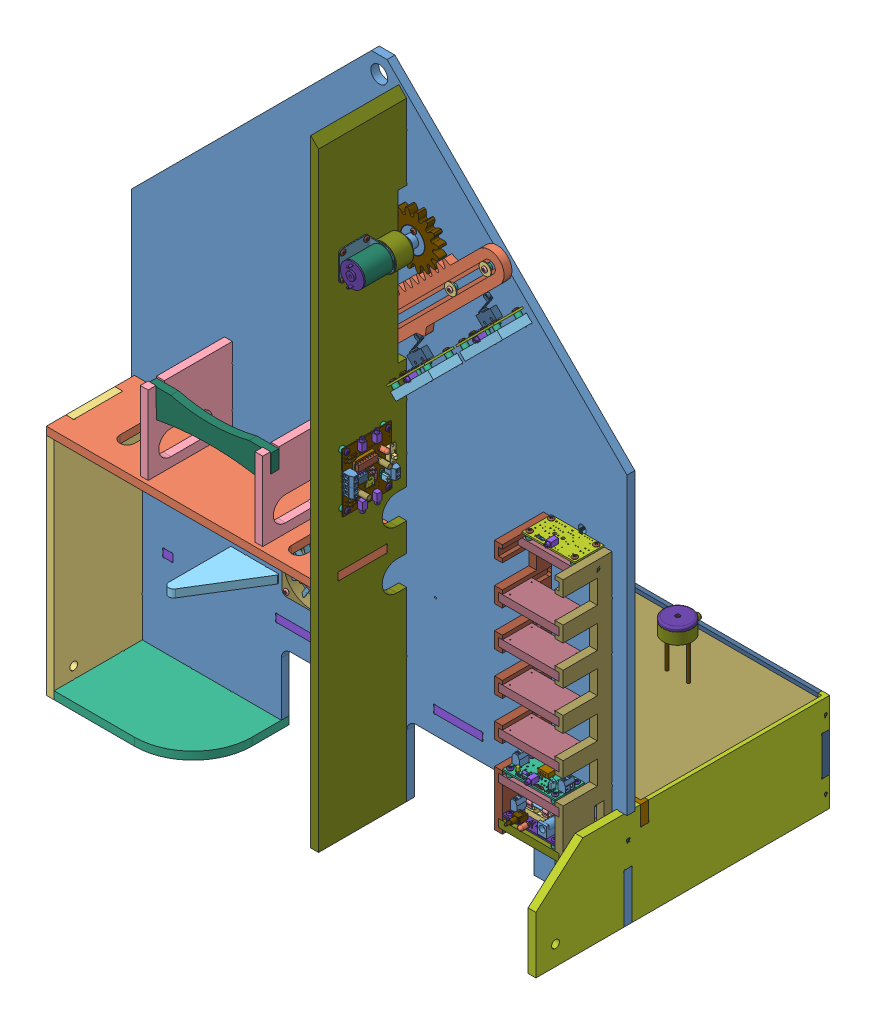
SolidWorks assembly Serre de base, configuration guillotine. Lengths in mm.
Overall size (506 646.24 310).
353 component instances, 97 part files, 150 mates.
Components (placement in the parent):
- FONDINTERIEUR-1: FONDINTERIEUR [Défaut] at (-62.876 -300.5478 -4)
- Crémallière M3-3-1: Crémallière M3-3 [Défaut] at (-39.5374 94.1308 4) x (0.707107 0.707107 0) z (0 0 1)
- Rondelle métal 3 x 12-1: Rondelle métal 3 x 12 [Défaut] at (57.939 191.6778 8)
- VIs TC 3 x 13-1: VIs TC 3 x 13 [Défaut] at (57.939 191.6778 2.4) x (1 0 0) z (0 -1 0)
- VIs TC 3 x 13-2: VIs TC 3 x 13 [Défaut] at (22.5836 156.3225 2.4) x (1 0 0) z (0 -1 0)
- Rondelle métal 3 x 12-2: Rondelle métal 3 x 12 [Défaut] at (22.5836 156.3225 8)
- Prépa 06 module Microrupteur-1: Prépa 06 module Microrupteur [Défaut] at (80.8247 148.8026 12.3834) x (0.707107 0.707107 0) z (-0.707107 0.707107 0) size (54 40.91 35.34)
  - support capteur-1: support capteur [Défaut] at (85.4284 22.7312 -4) size (54 38 8)
  - Entretoise CI-1: Entretoise CI [Défaut] at (-25.3985 -17.6166 4) size (5.9 5.9 4.1)
  - Entretoise CI-2: Entretoise CI [Défaut] at (-25.3985 4.3834 4) size (5.9 5.9 4.1)
  - Entretoise CI-3: Entretoise CI [Défaut] at (20.6015 -17.6166 4) size (5.9 5.9 4.1)
  - Entretoise CI-4: Entretoise CI [Défaut] at (20.6015 4.3834 4) size (5.9 5.9 4.1)
  - Module Microrupteur K-AP-MMR-1: Module Microrupteur K-AP-MMR [Défaut] at (24.602 -8.2581 10.6485) x (0 1 0) z (1 0 0) size (32.91 28.24 54)
    - CI-AP-MLBP avec jack-1: CI-AP-MLBP avec jack [Défaut] at (1.5279 -1.3102 0) size (32.91 8.01 54)
      - CI BP et DEL-1: CI BP et DEL [Défaut] at (-14.8869 -1.2382 0) size (30 1.6 54)
      - Embase jack 2.5-1: Embase jack 2.5 [Défaut] at (-14.8868 -1.2382 -27.0002) x (1 0 0) z (0 0 -1) size (10.81 8.01 5)
    - Résistance 10 K pas 11-1: Résistance 10 K pas 11 [Défaut] at (-6.8591 0.4515 -37.4997) x (0 0 -1) z (1 0 0) size (11.5 4.15 2.3)
    - Microrupteur-1: Microrupteur [Défaut] at (16.351 0.0515 -46.78) x (-1 0 0) z (0 0 -1) size (6.3 24.64 22.46)
  - VIs TC 3 x 6.5-1: VIs TC 3 x 6.5 [Défaut] at (-25.3985 -17.6166 3.3) x (1 0 0) z (0 -1 0) size (5.6 8.09 5.6)
  - VIs TC 3 x 6.5-2: VIs TC 3 x 6.5 [Défaut] at (-25.3979 4.3824 3.3) x (1 0 0) z (0 -1 0) size (5.6 8.09 5.6)
  - VIs TC 3 x 6.5-3: VIs TC 3 x 6.5 [Défaut] at (20.6015 -17.6166 3.3) x (0.418214 0.908348 0) z (0.908348 -0.418214 0) size (5.6 8.09 5.6)
  - VIs TC 3 x 6.5-4: VIs TC 3 x 6.5 [Défaut] at (20.6015 4.3834 3.3) x (1 0 0) z (0 -1 0) size (5.6 8.09 5.6)
- Prépa 06 module Microrupteur-2: Prépa 06 module Microrupteur [Défaut] at (10.114 78.0919 12.3834) x (0.707107 0.707107 0) z (-0.707107 0.707107 0) size (54 40.91 35.34)
  - support capteur-1: support capteur [Défaut] at (85.4284 22.7312 -4) size (54 38 8)
  - Entretoise CI-1: Entretoise CI [Défaut] at (-25.3985 -17.6166 4) size (5.9 5.9 4.1)
  - Entretoise CI-2: Entretoise CI [Défaut] at (-25.3985 4.3834 4) size (5.9 5.9 4.1)
  - Entretoise CI-3: Entretoise CI [Défaut] at (20.6015 -17.6166 4) size (5.9 5.9 4.1)
  - Entretoise CI-4: Entretoise CI [Défaut] at (20.6015 4.3834 4) size (5.9 5.9 4.1)
  - Module Microrupteur K-AP-MMR-1: Module Microrupteur K-AP-MMR [Défaut] at (24.602 -8.2581 10.6485) x (0 1 0) z (1 0 0) size (32.91 28.24 54)
    - CI-AP-MLBP avec jack-1: CI-AP-MLBP avec jack [Défaut] at (1.5279 -1.3102 0) size (32.91 8.01 54)
      - CI BP et DEL-1: CI BP et DEL [Défaut] at (-14.8869 -1.2382 0) size (30 1.6 54)
      - Embase jack 2.5-1: Embase jack 2.5 [Défaut] at (-14.8868 -1.2382 -27.0002) x (1 0 0) z (0 0 -1) size (10.81 8.01 5)
    - Résistance 10 K pas 11-1: Résistance 10 K pas 11 [Défaut] at (-6.8591 0.4515 -37.4997) x (0 0 -1) z (1 0 0) size (11.5 4.15 2.3)
    - Microrupteur-1: Microrupteur [Défaut] at (16.351 0.0515 -46.78) x (-1 0 0) z (0 0 -1) size (6.3 24.64 22.46)
  - VIs TC 3 x 6.5-1: VIs TC 3 x 6.5 [Défaut] at (-25.3985 -17.6166 3.3) x (1 0 0) z (0 -1 0) size (5.6 8.09 5.6)
  - VIs TC 3 x 6.5-2: VIs TC 3 x 6.5 [Défaut] at (-25.3979 4.3824 3.3) x (1 0 0) z (0 -1 0) size (5.6 8.09 5.6)
  - VIs TC 3 x 6.5-3: VIs TC 3 x 6.5 [Défaut] at (20.6015 -17.6166 3.3) x (0.418214 0.908348 0) z (0.908348 -0.418214 0) size (5.6 8.09 5.6)
  - VIs TC 3 x 6.5-4: VIs TC 3 x 6.5 [Défaut] at (20.6015 4.3834 3.3) x (1 0 0) z (0 -1 0) size (5.6 8.09 5.6)
- Ventilateur-1: Ventilateur [Défaut] at (-116.5864 -162.967 9.2) size (60 60 10.4)
  - Cage ventilateur-1: Cage ventilateur [Défaut] at (-27.2896 -30.9986 -5.2) size (60 60 10.4)
  - Hélice-1: Hélice [Défaut] at (3.0209 -0.9986 1.3) x (1 0 0) z (0 -1 0) size (55.32 5 55.41)
    - centre hélice-1: centre hélice [Défaut] at (-0.3105 -2.5 0) size (28.6 5 28.6)
    - Pale-1: Pale [Défaut] at (12.924 -1.982 -2.4379) x (-0.128403 0.431224 -0.893061) z (-0.06137 -0.902245 -0.426835) size (5.38 14.29 1.25)
    - Pale-12: Pale [Défaut] at (12.1411 -1.982 5.1043) x (0.374806 0.431224 -0.820711) z (0.179137 -0.902245 -0.392255) size (5.38 14.29 1.25)
    - Pale-13: Pale [Défaut] at (7.4049 -1.982 11.0258) x (0.759017 0.431224 -0.48779) z (0.362769 -0.902245 -0.233137) size (5.38 14.29 1.25)
    - Pale-14: Pale [Défaut] at (0.2191 -1.982 13.4468) x (0.902245 0.431224 0) z (0.431224 -0.902245 0) size (5.38 14.29 1.25)
    - Pale-15: Pale [Défaut] at (-7.1349 -1.982 11.5985) x (0.759017 0.431224 0.48779) z (0.362769 -0.902245 0.233137) size (5.38 14.29 1.25)
    - Pale-16: Pale [Défaut] at (-12.3221 -1.982 6.0677) x (0.374806 0.431224 0.820711) z (0.179137 -0.902245 0.392255) size (5.38 14.29 1.25)
    - Pale-17: Pale [Défaut] at (-13.6958 -1.982 -1.3895) x (-0.128403 0.431224 0.893061) z (-0.06137 -0.902245 0.426835) size (5.38 14.29 1.25)
    - Pale-18: Pale [Défaut] at (-10.8197 -1.982 -8.4055) x (-0.590845 0.431224 0.681871) z (-0.282392 -0.902245 0.325897) size (5.38 14.29 1.25)
    - Pale-19: Pale [Défaut] at (-4.6071 -1.982 -12.7529) x (-0.865698 0.431224 0.254192) z (-0.413756 -0.902245 0.12149) size (5.38 14.29 1.25)
    - Pale-20: Pale [Défaut] at (2.9697 -1.982 -13.0513) x (-0.865698 0.431224 -0.254192) z (-0.413756 -0.902245 -0.12149) size (5.38 14.29 1.25)
    - Pale-21: Pale [Défaut] at (9.505 -1.982 -9.206) x (-0.590845 0.431224 -0.681871) z (-0.282392 -0.902245 -0.325897) size (5.38 14.29 1.25)
- VIs TC 3 x 13-4: VIs TC 3 x 13 [Défaut] at (-138.876 -138.9656 8) x (1 0 0) z (0 -1 0)
- VIs TC 3 x 13-6: VIs TC 3 x 13 [Défaut] at (-88.876 -138.9656 8) x (1 0 0) z (0 -1 0)
- VIs TC 3 x 13-7: VIs TC 3 x 13 [Défaut] at (-88.876 -188.9656 8) x (1 0 0) z (0 -1 0)
- VIs TC 3 x 13-8: VIs TC 3 x 13 [Défaut] at (-138.876 -188.9656 8) x (1 0 0) z (0 -1 0)
- Entretoise CI-1: Entretoise CI [Défaut] at (57.939 191.6778 4) x (-0.97677 0.214292 0) z (0 0 1) size (5.9 5.9 4.1)
- Entretoise CI-2: Entretoise CI [Défaut] at (22.5836 156.3225 4) size (5.9 5.9 4.1)
- VIS TORCX TF 3 X 19-1: VIS TORCX TF 3 X 19 [Défaut] at (79.1287 147.1066 -4) x (-0.923728 -0.383049 0) z (0 0 -1)
- VIS TORCX TF 3 X 19-2: VIS TORCX TF 3 X 19 [Défaut] at (8.418 76.3959 -4) x (-0.923728 -0.383049 0) z (0 0 -1)
- Prépa 02 renfort arrière-1: Prépa 02 renfort arrière [Défaut] at (-30.876 -5.636 -123.7404) x (0 0 -1) z (1 0 0) size (98 630.07 61.8)
  - renfortarriere-1: renfortarriere [Défaut] at (-133.6202 -294.9118 -4) size (98 630.07 8)
  - Entretoise CI-1: Entretoise CI [Défaut] at (-194.2138 26.8323 4) size (5.9 5.9 4.1)
  - Entretoise CI-2: Entretoise CI [Défaut] at (-152.2157 27.0837 4) size (5.9 5.9 4.1)
  - Entretoise CI-3: Entretoise CI [Défaut] at (-193.9025 -25.1656 4) size (5.9 5.9 4.1)
  - Entretoise CI-4: Entretoise CI [Défaut] at (-151.9044 -24.9142 4) size (5.9 5.9 4.1)
  - VIs TC 3 x 9-1: VIs TC 3 x 9 [Défaut] at (-194.2138 26.8323 2.7) x (1 0 0) z (0 -1 0) size (5.6 10.69 5.6)
  - VIs TC 3 x 9-2: VIs TC 3 x 9 [Défaut] at (-152.2157 27.0837 2.7) x (1 0 0) z (0 -1 0) size (5.6 10.69 5.6)
  - VIs TC 3 x 9-3: VIs TC 3 x 9 [Défaut] at (-151.9044 -24.9142 2.7) x (1 0 0) z (0 -1 0) size (5.6 10.69 5.6)
  - VIs TC 3 x 9-4: VIs TC 3 x 9 [Défaut] at (-193.9025 -25.1656 2.7) x (1 0 0) z (0 -1 0) size (5.6 10.69 5.6)
  - Module 2 moteurs K-AP-MMOT-1: Module 2 moteurs K-AP-MMOT [Défaut] at (-148.0718 3.1444 10.7771) x (-0.005986 0.999982 0) z (0.999982 0.005986 0) size (65.82 19.5 50.56)
    - CI moteur-1: CI moteur [Défaut] at (-32.0357 -2.6771 0) size (60 1 50)
    - BORNIER 2-1: BORNIER 2 [Default] at (-17.0423 -1.6771 0.2294) x (0.999982 0 0.005986) z (0 1 0) size (9.97 7.55 15.02)
    - DEL D5 R-1: DEL D5 R [Défaut] at (9.6889 6.8229 -10.9906) x (1 0 0) z (0 -1 0) size (5.3 5.6 11.5)
    - Embase jack 2.5-1: Embase jack 2.5 [Défaut] at (-32.0356 -1.6771 -17.5006) size (10.81 8.01 5)
    - MICRO INVERSEUR A GLISSIERE-1: MICRO INVERSEUR A GLISSIERE [Défaut] at (3.55 3.3429 -4.0189) x (1 0 0.000537) z (0 1 0) size (19 5.82 12.15)
    - Résistance 220 ohm pas 11-1: Résistance 220 ohm pas 11 [Défaut] at (-10.0359 0.3229 -18.1991) x (-1 0 0) z (0 0 -1) size (11.5 4.15 2.3)
    - Embase jack 2.5-2: Embase jack 2.5 [Défaut] at (-32.0356 -1.6771 -32.5018) size (10.81 8.01 5)
    - Embase jack 2.5-3: Embase jack 2.5 [Défaut] at (27.964 -1.6771 -17.4981) x (-1 0 0) z (0 0 -1) size (10.81 8.01 5)
    - Embase jack 2.5-4: Embase jack 2.5 [Défaut] at (27.964 -1.6771 -32.4993) x (-1 0 0) z (0 0 -1) size (10.81 8.01 5)
    - Capuchon picot-1: Capuchon picot [Défaut] at (-16.1457 0.4729 -12.7155) x (1 0 0) z (0 -1 0) size (5.05 2.51 6.1)
    - ASB 3PICOTS-1: ASB 3PICOTS [Default] at (-9.9569 2.4259 -10.7946) x (1 0 0) z (0 -1 0) size (7.59 2.51 10)
      - PICOT-1: PICOT [Default] at (26.8516 -23.7306 1.953) size (2.51 2.51 10)
      - PICOT-2: PICOT [Default] at (29.3916 -23.7306 1.953) size (2.51 2.51 10)
      - PICOT-3: PICOT [Default] at (24.3116 -23.7306 1.953) size (2.51 2.51 10)
    - AJUSTABLE H-1: AJUSTABLE H [Défaut] at (-15.4716 0.3229 -24.988) x (0 0 1) z (0 1 0) size (8.6 10.76 7.4)
    - BORNIER 2-2: BORNIER 2 [Default] at (-2.0505 -1.6771 -50.2748) x (-1 0 0) z (0 1 0) size (9.97 7.55 15.02)
    - BORNIER 2-3: BORNIER 2 [Default] at (7.9495 -1.6771 -50.2748) x (-1 0 0) z (0 1 0) size (9.97 7.55 15.02)
    - Résistance 10 K pas 11-1: Résistance 10 K pas 11 [Défaut] at (19.1656 0.3229 -42.727) x (0 0 -1) z (1 0 0) size (11.5 4.15 2.3)
    - Résistance 10 K pas 11-2: Résistance 10 K pas 11 [Défaut] at (15.6274 0.3229 -42.6914) x (0 0 -1) z (1 0 0) size (11.5 4.15 2.3)
    - Résistance 10 K pas 11-3: Résistance 10 K pas 11 [Défaut] at (-19.5364 0.3229 -42.0005) x (0 0 -1) z (1 0 0) size (11.5 4.15 2.3)
    - Résistance 10 K pas 11-4: Résistance 10 K pas 11 [Défaut] at (-23.0365 0.3229 -42.0005) x (0 0 -1) z (1 0 0) size (11.5 4.15 2.3)
    - Support CI 8 pattes-1: Support CI 8 pattes [Défaut] at (-2.7368 -1.6771 -30.0083) x (0 0 -1) z (1 0 0) size (10 6 10.1)
    - Support CI 16 pattes-1: Support CI 16 pattes [Défaut] at (8.6068 -1.6771 -19.8458) x (0 0 -1) z (1 0 0) size (20.1 6 10.1)
    - CI 8 pattes-1: CI 8 pattes [Défaut] at (-2.7368 1.3229 -30.0113) x (0 0 -1) z (1 0 0) size (10 7.2 7.8)
    - CI 16 pattes-1: CI 16 pattes [Défaut] at (8.6068 1.3229 -19.8488) x (0 0 -1) z (1 0 0) size (20.1 7.2 7.8)
    - Capa 16V 100F 2.54-1: Capa 16V 100F 2.54 [Default] at (-14.0347 -26.6935 -37.5006) x (0 0 1) z (-1 0 0) size (5.2 15.5 5.88)
    - Capa 16V 100F 2.54-2: Capa 16V 100F 2.54 [Default] at (2.9618 -26.6935 -15.9995) x (0.999999 0 0.001464) z (-0.001464 0 0.999999) size (5.2 15.5 5.88)
    - condensateur 100nF-1: condensateur 100nF [Default] at (-2.9304 -7.4359 -15.4031) x (0 0 -1) z (1 0 0) size (5.85 10.35 1.99)
    - condensateur 100nF-2: condensateur 100nF [Default] at (0.5738 -7.4359 -15.3738) x (0 0 -1) z (1 0 0) size (5.85 10.35 1.99)
  - Moteur MFA 12-24V-1: Moteur MFA 12-24V [Défaut] at (-181.5572 189.3895 16.5047) x (-1 0 0) z (0 1 0) size (70.4 27.9 30)
    - Support moteur-1: Support moteur [Défaut] at (-14.3868 -12.5047 0) size (31 26.4 30)
    - Corps moteur-1: Corps moteur [Défaut] at (14.8132 1.8953 0) x (0 0 1) z (-1 0 0) size (24 24 63.9)
    - Capuchon moteur-1: Capuchon moteur [Défaut] at (-15.3868 1.8953 0) x (0 0 1) z (-1 0 0) size (27 27 18.7)
    - Arrière moteur-1: Arrière moteur [Défaut] at (16.3132 1.8953 0) x (0 0 1) z (-1 0 0) size (24 24 6.5)
  - Prépa 01 roue dentée-1: Prépa 01 roue dentée [Défaut] at (-131.9704 192.8178 10.3013) x (0 0.156764 -0.987636) z (1 0 0) size (54 54 14)
    - roue dentée 16-1: roue dentée 16 [Défaut] at (-7.1573 -1.556 -4) size (54 54 8)
    - Bague d'arrêt 4x12x24-1: Bague d'arrêt 4x12x24 [Défaut] at (-8.536 -2.1164 -10) x (0 1 0) z (0 0 1) size (24 24 8)
    - VIs TC 3 x 6.5-1: VIs TC 3 x 6.5 [Défaut] at (-8.536 6.8836 2.4) x (1 0 0) z (0 1 0) size (5.6 8.09 5.6)
    - VIs TC 3 x 6.5-2: VIs TC 3 x 6.5 [Défaut] at (-8.536 -11.1164 2.4) x (1 0 0) z (0 1 0) size (5.6 8.09 5.6)
  - VIs TC 3 x 6.5-1: VIs TC 3 x 6.5 [Défaut] at (-194.1704 201.3895 -1.4) x (1 0 0) z (0 -1 0) size (5.6 8.09 5.6)
  - VIs TC 3 x 6.5-2: VIs TC 3 x 6.5 [Défaut] at (-170.1704 201.3895 -1.4) x (1 0 0) z (0 -1 0) size (5.6 8.09 5.6)
  - VIs TC 3 x 6.5-3: VIs TC 3 x 6.5 [Défaut] at (-194.1704 177.3895 -1.4) x (1 0 0) z (0 -1 0) size (5.6 8.09 5.6)
  - VIs TC 3 x 6.5-4: VIs TC 3 x 6.5 [Défaut] at (-170.1704 177.3895 -1.4) x (1 0 0) z (0 -1 0) size (5.6 8.09 5.6)
- étagèrebrumi-1: étagèrebrumi [Défaut] at (-62.876 -93.9656 245.3364) x (1 0 0) z (0 1 0)
- VIS TORCX TF 3 X 19-3: VIS TORCX TF 3 X 19 [Défaut] at (-30.876 -315.9656 -4) x (-0.991079 -0.133274 0) z (0 0 -1)
- VIS TORCX TF 3 X 19-4: VIS TORCX TF 3 X 19 [Défaut] at (-30.876 -274.5499 -4) x (-0.991079 -0.133274 0) z (0 0 -1)
- VIS TORCX TF 3 X 19-5: VIS TORCX TF 3 X 19 [Défaut] at (-169.876 -89.9656 -4) x (-0.991079 -0.133274 0) z (0 0 -1)
- VIS TORCX TF 3 X 19-6: VIS TORCX TF 3 X 19 [Défaut] at (-30.876 -27.0369 -4) x (-0.991079 -0.133274 0) z (0 0 -1)
- VIS TORCX TF 3 X 19-7: VIS TORCX TF 3 X 19 [Défaut] at (-30.876 278.5344 -4) x (-0.991079 -0.133274 0) z (0 0 -1)
- Coté gauche serre-1: Coté gauche serre [Défaut] at (-304.876 -288.0405 43.9648) x (0 0 -1) z (1 0 0)
- Coté support brumisateur-1: Coté support brumisateur [Défaut] at (-87.876 -76.5368 52.2063) x (0 0 1) z (-1 0 0)
- Coté support brumisateur-2: Coté support brumisateur [Défaut] at (-204.876 -76.5368 52.2063) x (0 0 1) z (-1 0 0)
- Renfort bidon-1: Renfort bidon [Défaut] at (-206.376 -195.9656 85) x (1 0 0) z (0 1 0)
- suportbloceau-1: suportbloceau [Défaut] at (-238.3888 -323.9656 72.4161) x (1 0 0) z (0 1 0)
- VIS TORCX TF 3 X 19-12: VIS TORCX TF 3 X 19 [Défaut] at (-198.876 -191.9656 -4) x (-0.923728 -0.383049 0) z (0 0 -1)
- VIS TORCX TF 3 X 19-13: VIS TORCX TF 3 X 19 [Défaut] at (-164.4919 -191.9656 -4) x (-0.923728 -0.383049 0) z (0 0 -1)
- VIS TORCX TF 3 X 19-14: VIS TORCX TF 3 X 19 [Défaut] at (-208.876 -75.9656 -4) x (-0.923728 -0.383049 0) z (0 0 -1)
- VIS TORCX TF 3 X 19-15: VIS TORCX TF 3 X 19 [Défaut] at (-208.876 -16.4656 -4) x (-0.923728 -0.383049 0) z (0 0 -1)
- VIS TORCX TF 3 X 19-16: VIS TORCX TF 3 X 19 [Défaut] at (-91.876 -75.9656 -4) x (-0.923728 -0.383049 0) z (0 0 -1)
- VIS TORCX TF 3 X 19-17: VIS TORCX TF 3 X 19 [Défaut] at (-91.876 -15.9656 -4) x (-0.923728 -0.383049 0) z (0 0 -1)
- VIS TORCX TF 3 X 19-18: VIS TORCX TF 3 X 19 [Défaut] at (-304.876 -89.9656 48.9996) x (0 0 1) z (-1 0 0)
- VIS TORCX TF 3 X 19-25: VIS TORCX TF 3 X 19 [Défaut] at (-304.876 -248.9656 -0.0009) x (0 0 1) z (-1 0 0)
- VIS TORCX TF 3 X 19-26: VIS TORCX TF 3 X 19 [Défaut] at (-300.876 -323.9656 49) x (0.782535 0 -0.622606) z (0 -1 0)
- VIS TORCX TF 3 X 19-29: VIS TORCX TF 3 X 19 [Défaut] at (-271.876 -323.9656 0) x (0.782535 0 -0.622606) z (0 -1 0)
- VIS TORCX TF 3 X 19-30: VIS TORCX TF 3 X 19 [Défaut] at (-179.876 -323.9656 0) x (0.782535 0 -0.622606) z (0 -1 0)
- Coté droit serre-1: Coté droit serre [Défaut] at (187.124 -288.4466 43.9657) x (0 0 -1) z (1 0 0)
- VIS TORCX TF 3 X 19-35: VIS TORCX TF 3 X 19 [Défaut] at (195.124 -248.9656 0) x (0 -0.192039 -0.981387) z (1 0 0)
- Poutre fond-1: Poutre fond [Défaut] at (-62.876 -231.9656 64.5822) x (1 0 0) z (0 1 0)
- VIS TORCX TF 3 X 19-36: VIS TORCX TF 3 X 19 [Défaut] at (-213.1345 -227.9656 4)
- VIS TORCX TF 3 X 19-37: VIS TORCX TF 3 X 19 [Défaut] at (-54.876 -227.9656 4)
- Poutre plateau-1: Poutre plateau [Défaut] at (79.7388 -229.6404 -13) x (-1 0 0) z (0 0 -1)
- façadeporteplateau-1: façadeporteplateau [Défaut] at (102.5126 -276.3164 -206)
- VIS TORCX TF 3 X 19-38: VIS TORCX TF 3 X 19 [Défaut] at (191.124 -273.9656 -206) x (-0.923728 -0.383049 0) z (0 0 -1)
- VIS TORCX TF 3 X 19-39: VIS TORCX TF 3 X 19 [Défaut] at (195.124 -308.9656 -202) x (0 0 -1) z (1 0 0)
- VIS TORCX TF 3 X 19-40: VIS TORCX TF 3 X 19 [Défaut] at (195.124 -238.9656 -202) x (0 0 -1) z (1 0 0)
- VIS TORCX TF 3 X 19-43: VIS TORCX TF 3 X 19 [Défaut] at (-300.876 -273.9656 -206) x (-0.923728 -0.383049 0) z (0 0 -1)
- VIS TORCX TF 3 X 19-44: VIS TORCX TF 3 X 19 [Défaut] at (-304.876 -238.9737 -202) x (0 0 1) z (-1 0 0)
- VIS TORCX TF 3 X 19-45: VIS TORCX TF 3 X 19 [Défaut] at (-304.876 -308.9656 -202) x (0 0 1) z (-1 0 0)
- VIS TORCX TF 3 X 19-49: VIS TORCX TF 3 X 19 [Défaut] at (103.3825 -227.9656 4)
- Sous ensemble Rack module-1: Sous ensemble Rack module [Défaut] at (116.8547 -126.3174 -67.6389) x (0 0 -1) z (1 0 0) size (70.07 263.1 70)
  - rack coté gauche-1: rack coté gauche [Défaut] at (-102.2159 -95.6801 -4) size (58 256 8)
  - rack coté droit-1: rack coté droit [Défaut] at (-102.2159 -95.6628 58) size (58 256 8)
  - Prépa 05 module TEMP-1: Prépa 05 module TEMP [Défaut] at (-82.7846 122.513 33.0896) x (0 0 1) z (0 1 0) size (62 41.41 19.08)
    - supportcarterack-1: supportcarterack [Défaut] at (3.5074 9.0286 -6.1612) size (62 30 8)
    - Entretoise CI-1: Entretoise CI [Défaut] at (-25.0896 -14.8542 1.8388) size (5.9 5.9 4.1)
    - Entretoise CI-2: Entretoise CI [Défaut] at (-25.0896 7.1458 1.8388) size (5.9 5.9 4.1)
    - Entretoise CI-3: Entretoise CI [Défaut] at (20.9104 -14.8542 1.8388) size (5.9 5.9 4.1)
    - Entretoise CI-4: Entretoise CI [Défaut] at (20.9104 7.1458 1.8388) size (5.9 5.9 4.1)
    - Module temperature K-AP-MTEMP-1: Module temperature K-AP-MTEMP [Défaut] at (24.9109 -3.9678 7.1771) x (0 1 0) z (1 0 0) size (41.41 8.39 54)
      - CI BP et DEL-1: CI BP et DEL [Défaut] at (-14.8869 -1.2382 0) size (30 1.6 54)
      - Embase jack 2.5-1: Embase jack 2.5 [Défaut] at (-14.8868 0.3618 -27.0002) size (10.81 8.01 5)
      - Résistance 3,9 K pas 11-1: Résistance 3,9 K pas 11 [Défaut] at (-12.3875 1.7618 -37.4997) x (0 0 1) z (-1 0 0) size (11.5 4.15 2.3)
      - RC1 Tansistor plié 90°-1: RC1 Tansistor plié 90° [Défaut] at (18.6119 3.3399 -22.4989) x (0 0 -1) z (0 -1 0) size (4.8 10.25 6.98)
    - VIs TC 3 x 6.5-1: VIs TC 3 x 6.5 [Défaut] at (-25.0896 -14.8542 1.1388) x (1 0 0) z (0 -1 0) size (5.6 8.09 5.6)
    - VIs TC 3 x 6.5-2: VIs TC 3 x 6.5 [Défaut] at (-25.0896 7.1458 1.1388) x (1 0 0) z (0 -1 0) size (5.6 8.09 5.6)
    - VIs TC 3 x 6.5-3: VIs TC 3 x 6.5 [Défaut] at (20.9104 7.1458 1.1388) x (1 0 0) z (0 -1 0) size (5.6 8.09 5.6)
    - VIs TC 3 x 6.5-4: VIs TC 3 x 6.5 [Défaut] at (20.9104 -14.8542 1.1388) x (1 0 0) z (0 -1 0) size (5.6 8.09 5.6)
  - VIS TORCX TF 3 X 19-1: VIS TORCX TF 3 X 19 [Défaut] at (-86.6389 120.3518 66)
  - VIS TORCX TF 3 X 19-2: VIS TORCX TF 3 X 19 [Défaut] at (-86.6389 120.3431 -4) x (-0.923728 -0.383049 0) z (0 0 -1)
  - Prépa 04 module MAFU-1: Prépa 04 module MAFU [Défaut] at (-94.8752 -119.6656 28.2245) x (0 0 1) z (0 1 0) size (62 61.57 27.12)
    - basesuportpuissance-1: basesuportpuissance [Défaut] at (-4.8343 -1.5394 -4) size (62 50 8)
    - Entretoise CI-1: Entretoise CI [Défaut] at (-20.2245 -22.7636 4) size (5.9 5.9 4.1)
    - Entretoise CI-2: Entretoise CI [Défaut] at (-20.2245 -0.7636 4) size (5.9 5.9 4.1)
    - Entretoise CI-3: Entretoise CI [Défaut] at (25.7755 -0.7636 4) size (5.9 5.9 4.1)
    - Entretoise CI-4: Entretoise CI [Défaut] at (25.7755 -22.7636 4) size (5.9 5.9 4.1)
    - CI-MAFU avec borniers-1: CI-MAFU avec borniers [Défaut] at (2.9088 -18.7288 8.9) x (0 -1 0) z (0 0 1) size (43.65 55.05 18.42)
      - CI-MAFU-1: CI-MAFU [Défaut] at (-21.9652 -27.1333 -0.8) size (30 54 1.6)
      - Inter long à souder 734-7220-1: Inter long à souder 734-7220 [Défaut] at (8.1051 -9.1203 1.3) x (-1 0 0) z (0 1 0) size (20.8 9.2 8)
      - Embase femelle d'alimentation-1: Embase femelle d'alimentation [Défaut] at (4.7338 12.8853 0.8) x (0 -1 0) z (-1 0 0) size (10.39 15 14.1)
      - DEL D5 rouge pliée-2: DEL D5 rouge pliée [Défaut] at (17.5325 -1.131 5.2) x (0 1 0) z (-1 0 0) size (5.3 8.8 12.9)
      - Support fusible avec fusible-1: Support fusible avec fusible [Défaut] at (-8.3615 -5.1853 4.8987) x (0 1 0) z (1 0 0) size (23 17 8.6)
        - Support fusible base-1: Support fusible base [Défaut] at (-10.9359 -4.0987 -4.3) size (22 7 8.6)
        - Support fusible contact-1: Support fusible contact [Défaut] at (5.4641 0.8731 -0.0014) size (6.1 17 6.2)
        - Support fusible contact-2: Support fusible contact [Défaut] at (-5.3359 0.8731 -0.0014) x (-1 0 0) z (0 0 -1) size (6.1 17 6.2)
        - Fusible-1: Fusible [Défaut] at (-0.0359 6.2731 -0.0014) size (19.8 5.2 5.2)
      - BORNIER 2-2: BORNIER 2 [Default] at (-24.0402 -10.1483 0.8) x (0 -1 0) z (0 0 1) size (9.97 7.55 15.02)
      - BORNIER 2-4: BORNIER 2 [Default] at (-24.0402 -0.1483 0.8) x (0 -1 0) z (0 0 1) size (9.97 7.55 15.02)
      - BORNIER 2-5: BORNIER 2 [Default] at (-24.0402 9.8517 0.8) x (0 -1 0) z (0 0 1) size (9.97 7.55 15.02)
      - BORNIER 2-6: BORNIER 2 [Default] at (-24.0402 19.8517 0.8) x (0 -1 0) z (0 0 1) size (9.97 7.55 15.02)
      - BORNIER 2-7: BORNIER 2 [Default] at (-10.2502 -27.9083 0.8) size (9.97 7.55 15.02)
      - BORNIER 2-9: BORNIER 2 [Default] at (-0.2802 27.1417 0.8) x (-1 0 0) z (0 0 1) size (9.97 7.55 15.02) (hidden)
    - VIs TC 3 x 9-1: VIs TC 3 x 9 [Défaut] at (-20.2245 -22.7636 3.3) x (1 0 0) z (0 -1 0) size (5.6 10.69 5.6)
    - VIs TC 3 x 9-2: VIs TC 3 x 9 [Défaut] at (25.7755 -22.7636 3.3) x (1 0 0) z (0 -1 0) size (5.6 10.69 5.6)
    - VIs TC 3 x 9-3: VIs TC 3 x 9 [Défaut] at (-20.2245 -0.7636 3.3) x (1 0 0) z (0 -1 0) size (5.6 10.69 5.6)
    - VIs TC 3 x 9-4: VIs TC 3 x 9 [Défaut] at (25.7755 -0.7636 3.3) x (1 0 0) z (0 -1 0) size (5.6 10.69 5.6)
  - VIS TORCX TF 3 X 19-3: VIS TORCX TF 3 X 19 [Défaut] at (-107.1389 -119.6824 66)
  - VIS TORCX TF 3 X 19-4: VIS TORCX TF 3 X 19 [Défaut] at (-78.1389 -119.6824 66)
  - VIS TORCX TF 3 X 19-6: VIS TORCX TF 3 X 19 [Défaut] at (-107.1389 -119.6656 -4) x (-0.923728 -0.383049 0) z (0 0 -1)
  - VIS TORCX TF 3 X 19-7: VIS TORCX TF 3 X 19 [Défaut] at (-78.1389 -119.6656 -4) x (-0.923728 -0.383049 0) z (0 0 -1)
  - Prépa 03 module PWR-1: Prépa 03 module PWR [Défaut] at (-104.636 -79.6656 32.1892) x (0 0 1) z (0 1 0) size (62 33.06 23.72)
    - supportcarterack-1: supportcarterack [Défaut] at (4.4079 10.88 -4) size (62 30 8)
    - Entretoise CI-1: Entretoise CI [Défaut] at (-24.1892 -13.0028 4) size (5.9 5.9 4.1)
    - Entretoise CI-2: Entretoise CI [Défaut] at (-24.1892 8.9972 4) size (5.9 5.9 4.1)
    - Entretoise CI-3: Entretoise CI [Défaut] at (21.8108 8.9972 4) size (5.9 5.9 4.1)
    - Entretoise CI-4: Entretoise CI [Défaut] at (21.8108 -13.0028 4) size (5.9 5.9 4.1)
    - Module K-AP-MPWR-1: Module K-AP-MPWR [Défaut] at (-1.2571 1.9363 8.9) x (0 1 0) z (0 0 1) size (33.06 54.47 15.02)
      - CI AP-PWR-1: CI AP-PWR [Défaut] at (-18.9391 -27.0679 -0.8) size (30 54 1.6)
      - BORNIER 2-1: BORNIER 2 [Default] at (0.963 27.1235 0.8) x (-1 0 0) z (0 0 1) size (9.97 7.55 15.02)
      - DELverte 3mm-1: DELverte 3mm [Défaut] at (-12.9358 16.93 1.8) x (0 0 1) z (-1 0 0) size (7.4 3.42 3.8)
      - diode-1: diode [Défaut] at (-12.9396 11.4315 3.2) x (1 0 0) z (0 -1 0) size (2.65 5.32 8.12)
      - ASB 3PICOTS avec capuchon-1: ASB 3PICOTS avec capuchon [Default] at (-16.084 -16.9024 4.903) x (-1 0 0) z (0 0 -1) size (7.59 2.51 10.25)
        - PICOT-1: PICOT [Default] at (26.8516 -23.7306 1.953) size (2.51 2.51 10)
        - PICOT-2: PICOT [Default] at (29.3916 -23.7306 1.953) size (2.51 2.51 10)
        - PICOT-3: PICOT [Default] at (24.3116 -23.7306 1.953) size (2.51 2.51 10)
        - Capuchon picot-1: Capuchon picot [Défaut] at (-6.1888 -1.9209 1.953) size (5.05 2.51 6.1)
      - Embase jack 2.5-1: Embase jack 2.5 [Défaut] at (-18.9403 -0.0677 0.8) x (1 0 0) z (0 -1 0) size (10.81 8.01 5)
      - REG-1: REG [Default] at (-4.2884 5.0073 0.8) x (0 -1 0) z (0 0 1) size (10.15 20.05 5.19)
      - Résistance 220 pas 11-1: Résistance 220 pas 11 [Défaut] at (-17.2386 9.3312 2.2) x (0 -1 0) z (-1 0 0) size (11.5 4.15 2.3)
      - Résistance 10K pas de 11-1: Résistance 10K pas de 11 [Défaut] at (-17.2386 -9.3683 2.2) x (0 -1 0) z (-1 0 0) size (11.5 4.15 2.3)
      - BORNIER 2-2: BORNIER 2 [Default] at (-8.9238 -27.3428 0.8) size (9.97 7.55 15.02)
    - VIs TC 3 x 9-1: VIs TC 3 x 9 [Défaut] at (-24.1892 -13.0028 3.3) x (1 0 0) z (0 -1 0) size (5.6 10.69 5.6)
    - VIs TC 3 x 9-2: VIs TC 3 x 9 [Défaut] at (-24.1892 8.9972 3.3) x (1 0 0) z (0 -1 0) size (5.6 10.69 5.6)
    - VIs TC 3 x 9-3: VIs TC 3 x 9 [Défaut] at (21.8108 8.9972 3.3) x (1 0 0) z (0 -1 0) size (5.6 10.69 5.6)
    - VIs TC 3 x 9-4: VIs TC 3 x 9 [Défaut] at (21.8108 -13.0028 3.3) x (1 0 0) z (0 -1 0) size (5.6 10.69 5.6)
  - supportcarterack-1: supportcarterack [Défaut] at (-119.5217 -35.6656 36.597) x (0 0 1) z (0 -1 0) size (62 30 8)
  - supportcarterack-2: supportcarterack [Défaut] at (-119.5217 4.3344 36.597) x (0 0 1) z (0 -1 0) size (62 30 8)
  - supportcarterack-3: supportcarterack [Défaut] at (-119.5217 44.3344 36.597) x (0 0 1) z (0 -1 0) size (62 30 8)
  - supportcarterack-4: supportcarterack [Défaut] at (-119.5217 84.3344 36.597) x (0 0 1) z (0 -1 0) size (62 30 8)
- VIS TORCX TF 3 X 19-50: VIS TORCX TF 3 X 19 [Défaut] at (178.8547 -145.9656 -4) x (-0.923728 -0.383049 0) z (0 0 -1)
- VIS TORCX TF 3 X 19-51: VIS TORCX TF 3 X 19 [Défaut] at (116.8547 -145.9656 -4) x (-0.923728 -0.383049 0) z (0 0 -1)
- VIS TORCX TF 3 X 19-52: VIS TORCX TF 3 X 19 [Défaut] at (178.8547 -7.9656 -4) x (-0.923728 -0.383049 0) z (0 0 -1)
- VIS TORCX TF 3 X 19-53: VIS TORCX TF 3 X 19 [Défaut] at (116.8547 -7.9656 -4) x (-0.923728 -0.383049 0) z (0 0 -1)
- Sous ensemble Arrosage-1: Sous ensemble Arrosage [Défaut] at (-248.1801 -261.6655 37.8651) x (-0.00308 0 0.999995) z (0 -1 0) size (140.54 240.54 274.35) (hidden)
  - Pompe-1: Pompe [Défaut] at (-9.0938 -0.5877 17.5) size (40 29 55)
  - Tuyau gouteur-1: Tuyau gouteur [Défaut] at (-69.6171 -162.8404 -195.5) x (0 0 -1) z (0.999995 -0.00308 0) size (203 173 86)
  - Gouteur-1: Gouteur [Défaut] at (-70.8858 -170.9803 -151.85) x (-0.999995 0.00308 0) z (0 0 1) size (21 26.3 133.2)
    - PiedGouteur-1: PiedGouteur [Défaut] at (-1.2437 2.6563 -65) size (16 23.8 130)
    - BouchonGouteur-1: BouchonGouteur [Défaut] at (-1.2437 2.6563 -57) x (-0.923728 -0.383049 0) z (0 0 -1) size (16.07 16.07 11.2)
  - Bouchon reservoir-1: Bouchon reservoir [Défaut] at (10.9062 6.9123 -125.7) x (0.574699 -0.818365 0) z (0.818365 0.574699 0) size (71 20 71)
  - Passe cable-1: Passe cable [Défaut] at (10.9062 6.9123 -169.9434) x (0 0 -1) z (0 1 0) size (6 11 11)
  - Reservoir 1,25L-1: Reservoir 1,25L [Défaut] at (7.3532 24.2973 -125.7) x (0.999995 -0.00308 0) z (0 0 1) size (89.5 89.5 187)
- plateau base-1: plateau base [Défaut] at (-230.7684 -235.9656 -41.3241) x (1 0 0) z (0 1 0)
- fondcuivré-1: fondcuivré [Défaut] at (-208.3657 -251.1382 -5)
- Capot complet-1: Capot complet [Vitres] at (-187.0166 -15.8593 -60) x (-1 0 0) z (0 0 -1) size (516 661.85 308) (hidden)
  - Capot coté droit-1: Capot coté droit [Défaut] at (-332.1697 -265.6526 -154) size (263.66 661.85 308)
  - Capot coté gauche-1: Capot coté gauche [Défaut] at (175.8303 -266.1888 -154) size (263.66 661.85 308)
  - Capotfaçade-1: Capotfaçade [Défaut] at (75.9652 -264.3201 154) x (-1 0 0) z (0 0 -1) size (516 661.85 8)
  - Vitre laterale-1: Vitre laterale [Défaut] at (-385.1406 -165.6883 102.4285) x (0 1 0) z (1 0 0) size (290.43 181.9 2)
  - Vitre avant grande-1: Vitre avant grande [Défaut] at (-355.6546 -169.3327 147) x (0 1 0) z (0 0 1) size (286.8 171.11 2)
  - Vitre laterale-2: Vitre laterale [Défaut] at (120.8594 30.4421 102.4285) x (0 -1 0) z (-1 0 0) size (290.43 181.9 2)
  - Vitre avant grande-2: Vitre avant grande [Défaut] at (-40.8684 -169.3327 147) x (0 1 0) z (0 0 1) size (286.8 171.11 2)
  - Vitre avant centrale-1: Vitre avant centrale [Défaut] at (-154.2178 43.2096 147) size (123.47 286.8 2)
  - Vitre laterale-4: Vitre laterale [Défaut] at (-65.085 276.7887 -22.3285) x (0.707107 -0.707107 0) z (0.707107 0.707107 0) size (290.43 181.9 2)
  - Charnière percée-1: Charnière percée [Défaut] at (-176.8635 321.0541 -74.2825) x (-0.707107 -0.707107 0) z (0 0 -1) size (25.5 17 19)
    - Charnière percée-1: Charnière percée [Défaut] at (-8.739 -12.0088 -9.5) size (11 16 19)
    - Charnièere percée  2-1: Charnièere percée  2 [Défaut] at (-8.739 1.9912 -4) size (25.5 13 19)
  - Charnière percée-2: Charnière percée [Défaut] at (-176.8635 321.0541 120.9123) x (-0.707107 -0.707107 0) z (0 0 -1) size (25.5 17 19)
    - Charnière percée-1: Charnière percée [Défaut] at (-8.739 -12.0088 -9.5) size (11 16 19)
    - Charnièere percée  2-1: Charnièere percée  2 [Défaut] at (-8.739 1.9912 -4) size (25.5 13 19)
  - VIS TORCX TF 3 X 13-4: VIS TORCX TF 3 X 13 [Défaut] at (-159.0106 315.56 -74.2825) x (0.5 0.5 -0.707107) z (0.707107 -0.707107 0) size (5.6 5.6 13)
  - VIS TORCX TF 3 X 13-5: VIS TORCX TF 3 X 13 [Défaut] at (-159.0106 315.56 120.9123) x (0.5 0.5 -0.707107) z (0.707107 -0.707107 0) size (5.6 5.6 13)
  - VIS TORCX TF 3 X 19-1: VIS TORCX TF 3 X 19 [Défaut] at (-386.1406 -283.1062 154)
  - VIS TORCX TF 3 X 19-2: VIS TORCX TF 3 X 19 [Défaut] at (-386.1406 -233.1062 154)
  - VIS TORCX TF 3 X 19-3: VIS TORCX TF 3 X 19 [Défaut] at (-386.1406 -125.6062 154)
  - VIS TORCX TF 3 X 19-4: VIS TORCX TF 3 X 19 [Défaut] at (-386.1406 -15.6062 154)
  - VIS TORCX TF 3 X 19-5: VIS TORCX TF 3 X 19 [Défaut] at (-386.1406 81.3179 154)
  - VIS TORCX TF 3 X 19-6: VIS TORCX TF 3 X 19 [Défaut] at (-376.7525 103.4731 154)
  - VIS TORCX TF 3 X 19-7: VIS TORCX TF 3 X 19 [Défaut] at (-307.8566 172.3691 154)
  - VIS TORCX TF 3 X 19-8: VIS TORCX TF 3 X 19 [Défaut] at (-230.0748 250.1508 154)
  - VIS TORCX TF 3 X 19-9: VIS TORCX TF 3 X 19 [Défaut] at (-150.5253 329.7003 154)
  - VIS TORCX TF 3 X 19-10: VIS TORCX TF 3 X 19 [Défaut] at (-134.969 350.9153 96) x (0.5 0.5 0.707107) z (-0.707107 0.707107 0)
  - VIS TORCX TF 3 X 19-11: VIS TORCX TF 3 X 19 [Défaut] at (-129.3121 350.9153 -4) x (0.5 -0.5 -0.707107) z (0.707107 0.707107 0)
  - VIS TORCX TF 3 X 19-22: VIS TORCX TF 3 X 19 [Défaut] at (-134.969 350.9153 -104) x (0.5 0.5 0.707107) z (-0.707107 0.707107 0)
  - VIS TORCX TF 3 X 19-24: VIS TORCX TF 3 X 19 [Défaut] at (-113.7558 329.7003 154)
  - VIS TORCX TF 3 X 19-25: VIS TORCX TF 3 X 19 [Défaut] at (-34.2063 250.1508 154)
  - VIS TORCX TF 3 X 19-26: VIS TORCX TF 3 X 19 [Défaut] at (43.5755 172.3691 154)
  - VIS TORCX TF 3 X 19-27: VIS TORCX TF 3 X 19 [Défaut] at (112.4714 103.4731 154)
  - VIS TORCX TF 3 X 19-28: VIS TORCX TF 3 X 19 [Défaut] at (121.8594 81.3179 154)
  - VIS TORCX TF 3 X 19-29: VIS TORCX TF 3 X 19 [Défaut] at (121.8594 -15.6062 154)
  - VIS TORCX TF 3 X 19-30: VIS TORCX TF 3 X 19 [Défaut] at (121.8594 -233.1062 154)
  - VIS TORCX TF 3 X 19-31: VIS TORCX TF 3 X 19 [Défaut] at (121.8594 -125.6062 154)
  - VIS TORCX TF 3 X 19-32: VIS TORCX TF 3 X 19 [Défaut] at (121.8594 -283.1062 154)
  - Aimant-1: Aimant [Défaut] at (122.8594 -288.1062 -134) x (0 0 1) z (-1 0 0) size (8 8 5)
  - Aimant-2: Aimant [Défaut] at (-387.1406 -288.1062 -134) x (0 0 -1) z (1 0 0) size (8 8 5)
  - VIS TF 2.2x6.4-114: VIS TF 2.2x6.4 [Défaut] at (-383.1406 75.3601 128.5) x (0 -1 0) z (1 0 0) size (4.2 4.2 6.4)
  - VIS TF 2.2x6.4-115: VIS TF 2.2x6.4 [Défaut] at (-383.1406 -67.3599 128.5) x (0 -1 0) z (1 0 0) size (4.2 4.2 6.4)
  - VIS TF 2.2x6.4-116: VIS TF 2.2x6.4 [Défaut] at (-383.1406 -210.0699 128.5) x (0 -1 0) z (1 0 0) size (4.2 4.2 6.4)
  - VIS TF 2.2x6.4-117: VIS TF 2.2x6.4 [Défaut] at (-383.2825 -210.0699 -48.4) x (0 -1 0) z (0 0 1) size (4.2 4.2 6.4)
  - VIS TF 2.2x6.4-118: VIS TF 2.2x6.4 [Défaut] at (-383.2825 -67.3599 -48.4) x (0 -1 0) z (0 0 1) size (4.2 4.2 6.4)
  - VIS TF 2.2x6.4-119: VIS TF 2.2x6.4 [Défaut] at (-383.2825 75.3601 -48.4) x (0 -1 0) z (0 0 1) size (4.2 4.2 6.4)
  - VIS TF 2.2x6.4-120: VIS TF 2.2x6.4 [Défaut] at (-372.6406 -210.6062 147) x (1 0 0) z (0 0 -1) size (4.2 4.2 6.4)
  - VIS TF 2.2x6.4-121: VIS TF 2.2x6.4 [Défaut] at (-206.5306 -210.6062 147) x (1 0 0) z (0 0 -1) size (4.2 4.2 6.4)
  - VIS TF 2.2x6.4-122: VIS TF 2.2x6.4 [Défaut] at (-191.4267 -210.6062 147) x (1 0 0) z (0 0 -1) size (4.2 4.2 6.4)
  - VIS TF 2.2x6.4-123: VIS TF 2.2x6.4 [Défaut] at (-72.9567 -210.6062 147) x (1 0 0) z (0 0 -1) size (4.2 4.2 6.4)
  - VIS TF 2.2x6.4-124: VIS TF 2.2x6.4 [Défaut] at (118.8594 -210.6062 128.5) x (0 1 0) z (-1 0 0) size (4.2 4.2 6.4)
  - VIS TF 2.2x6.4-125: VIS TF 2.2x6.4 [Défaut] at (-372.6406 -69.7062 147) x (1 0 0) z (0 0 -1) size (4.2 4.2 6.4)
  - VIS TF 2.2x6.4-126: VIS TF 2.2x6.4 [Défaut] at (-206.5306 -70.0886 147) x (1 0 0) z (0 0 -1) size (4.2 4.2 6.4)
  - VIS TF 2.2x6.4-127: VIS TF 2.2x6.4 [Défaut] at (-191.4267 -66.7062 147) x (1 0 0) z (0 0 -1) size (4.2 4.2 6.4)
  - VIS TF 2.2x6.4-128: VIS TF 2.2x6.4 [Défaut] at (-72.9567 -62.2592 147) x (1 0 0) z (0 0 -1) size (4.2 4.2 6.4)
  - VIS TF 2.2x6.4-129: VIS TF 2.2x6.4 [Défaut] at (118.8594 -67.8862 128.5) x (0 1 0) z (-1 0 0) size (4.2 4.2 6.4)
  - VIS TF 2.2x6.4-130: VIS TF 2.2x6.4 [Défaut] at (-372.6406 71.1938 147) x (-0.923728 -0.383049 0) z (0 0 -1) size (4.2 4.2 6.4)
  - VIS TF 2.2x6.4-131: VIS TF 2.2x6.4 [Défaut] at (-206.5306 71.1938 147) x (1 0 0) z (0 0 -1) size (4.2 4.2 6.4)
  - VIS TF 2.2x6.4-132: VIS TF 2.2x6.4 [Défaut] at (-191.4267 71.1938 147) x (-0.923728 -0.383049 0) z (0 0 -1) size (4.2 4.2 6.4)
  - VIS TF 2.2x6.4-133: VIS TF 2.2x6.4 [Défaut] at (-72.9567 71.1938 147) x (1 0 0) z (0 0 -1) size (4.2 4.2 6.4)
  - VIS TF 2.2x6.4-134: VIS TF 2.2x6.4 [Défaut] at (118.8594 74.8238 128.5) x (0 1 0) z (-1 0 0) size (4.2 4.2 6.4)
  - VIS TF 2.2x6.4-135: VIS TF 2.2x6.4 [Défaut] at (118.8594 74.8238 -48.4) x (0 1 0) z (-1 0 0) size (4.2 4.2 6.4)
  - VIS TF 2.2x6.4-136: VIS TF 2.2x6.4 [Défaut] at (118.8594 -67.8862 -48.4) x (0 1 0) z (-1 0 0) size (4.2 4.2 6.4)
  - VIS TF 2.2x6.4-137: VIS TF 2.2x6.4 [Défaut] at (118.8594 -210.6062 -48.4) x (0 1 0) z (-1 0 0) size (4.2 4.2 6.4)
  - VIS TF 2.2x6.4-138: VIS TF 2.2x6.4 [Défaut] at (-57.8544 -210.6062 147) x (1 0 0) z (0 0 -1) size (4.2 4.2 6.4)
  - VIS TF 2.2x6.4-139: VIS TF 2.2x6.4 [Défaut] at (108.2556 -210.6062 147) x (1 0 0) z (0 0 -1) size (4.2 4.2 6.4)
  - VIS TF 2.2x6.4-140: VIS TF 2.2x6.4 [Défaut] at (-57.8544 -69.7062 147) x (1 0 0) z (0 0 -1) size (4.2 4.2 6.4)
  - VIS TF 2.2x6.4-141: VIS TF 2.2x6.4 [Défaut] at (108.2556 -70.0886 147) x (1 0 0) z (0 0 -1) size (4.2 4.2 6.4)
  - VIS TF 2.2x6.4-142: VIS TF 2.2x6.4 [Défaut] at (-57.8544 71.1938 147) x (1 0 0) z (0 0 -1) size (4.2 4.2 6.4)
  - VIS TF 2.2x6.4-143: VIS TF 2.2x6.4 [Défaut] at (108.2556 71.1938 147) x (1 0 0) z (0 0 -1) size (4.2 4.2 6.4)
  - VIS TF 2.2x6.4-144: VIS TF 2.2x6.4 [Défaut] at (107.098 88.486 147) x (1 0 0) z (0 0 -1) size (4.2 4.2 6.4)
  - VIS TF 2.2x6.4-145: VIS TF 2.2x6.4 [Défaut] at (105.3619 106.3418 128.5) x (-0.707107 0.707107 0) z (-0.707107 -0.707107 0) size (4.2 4.2 6.4)
  - VIS TF 2.2x6.4-146: VIS TF 2.2x6.4 [Défaut] at (105.3619 106.3418 -48.4) x (-0.707107 0.707107 0) z (-0.707107 -0.707107 0) size (4.2 4.2 6.4)
  - VIS TF 2.2x6.4-147: VIS TF 2.2x6.4 [Défaut] at (-131.8128 86.5458 147) x (1 0 0) z (0 0 -1) size (4.2 4.2 6.4)
  - VIS TF 2.2x6.4-148: VIS TF 2.2x6.4 [Défaut] at (4.4436 207.2601 -48.4) x (-0.707107 0.707107 0) z (-0.707107 -0.707107 0) size (4.2 4.2 6.4)
  - VIS TF 2.2x6.4-149: VIS TF 2.2x6.4 [Défaut] at (-3.5291 201.728 147) x (1 0 0) z (0 0 -1) size (4.2 4.2 6.4)
  - VIS TF 2.2x6.4-150: VIS TF 2.2x6.4 [Défaut] at (-96.4676 308.1713 -48.4) x (-0.707107 0.707107 0) z (-0.707107 -0.707107 0) size (4.2 4.2 6.4)
  - VIS TF 2.2x6.4-151: VIS TF 2.2x6.4 [Défaut] at (-96.4676 308.1713 128.5) x (-0.707107 0.707107 0) z (-0.707107 -0.707107 0) size (4.2 4.2 6.4)
  - VIS TF 2.2x6.4-152: VIS TF 2.2x6.4 [Défaut] at (-131.8128 309.8158 147) x (1 0 0) z (0 0 -1) size (4.2 4.2 6.4)
  - VIS TF 2.2x6.4-153: VIS TF 2.2x6.4 [Défaut] at (4.4436 207.2601 128.5) x (-0.707107 0.707107 0) z (-0.707107 -0.707107 0) size (4.2 4.2 6.4)
  - VIS TF 2.2x6.4-154: VIS TF 2.2x6.4 [Défaut] at (-370.7236 88.486 147) x (1 0 0) z (0 0 -1) size (4.2 4.2 6.4)
  - VIS TF 2.2x6.4-155: VIS TF 2.2x6.4 [Défaut] at (-260.0965 201.728 147) x (1 0 0) z (0 0 -1) size (4.2 4.2 6.4)
  - Fenêtre complete-1: Fenêtre complete [Défaut] at (-268.7504 217.134 52.5771) x (0 0 1) z (-0.707107 0.707107 0) size (216 290.55 23)
    - Fenêtre-1: Fenêtre [Défaut] at (-151.0146 -563.7006 -4) size (216 290.55 8)
    - poignée fenetre-1: poignée fenetre [Défaut] at (-29.6647 -138.358 4) x (1 0 0) z (0 -1 0) size (200 15 8)
    - Vitre fenetre-1: Vitre fenetre [Défaut] at (-68.8332 -67.4201 -4) x (0 1 0) z (0 0 1) size (258.45 165.9 2)
    - VIS TF 2.2x6.4-15: VIS TF 2.2x6.4 [Défaut] at (60.7353 -134.7546 -4) x (-0.714663 -0.699469 0) z (0 0 -1) size (4.2 4.2 6.4)
    - VIS TF 2.2x6.4-16: VIS TF 2.2x6.4 [Défaut] at (60.7353 -8.0346 -4) x (-0.714663 -0.699469 0) z (0 0 -1) size (4.2 4.2 6.4)
    - VIS TF 2.2x6.4-17: VIS TF 2.2x6.4 [Défaut] at (60.7353 118.6954 -4) x (-0.714663 -0.699469 0) z (0 0 -1) size (4.2 4.2 6.4)
    - VIS TF 2.2x6.4-18: VIS TF 2.2x6.4 [Défaut] at (-100.1647 118.6954 -4) x (-0.714663 -0.699469 0) z (0 0 -1) size (4.2 4.2 6.4)
    - VIS TF 2.2x6.4-19: VIS TF 2.2x6.4 [Défaut] at (-100.1647 -8.0346 -4) x (-0.714663 -0.699469 0) z (0 0 -1) size (4.2 4.2 6.4)
    - VIS TF 2.2x6.4-20: VIS TF 2.2x6.4 [Défaut] at (-100.1647 -134.7546 -4) x (-0.714663 -0.699469 0) z (0 0 -1) size (4.2 4.2 6.4)
    - VIS TORCX TF 3 X 19-1: VIS TORCX TF 3 X 19 [Défaut] at (-101.3516 -142.358 -4) x (-0.923728 -0.383049 0) z (0 0 -1)
    - VIS TORCX TF 3 X 19-2: VIS TORCX TF 3 X 19 [Défaut] at (43.6484 -142.358 -4) x (-0.923728 -0.383049 0) z (0 0 -1)
  - VIS TORCX TF 3 X 13-1: VIS TORCX TF 3 X 13 [Défaut] at (-174.567 311.3174 120.9123) x (-0.355164 -0.355164 0.864706) z (0.707107 -0.707107 0) size (5.6 5.6 13)
  - VIS TORCX TF 3 X 13-2: VIS TORCX TF 3 X 13 [Défaut] at (-174.567 311.3174 -74.3702) x (-0.355164 -0.355164 0.864706) z (0.707107 -0.707107 0) size (5.6 5.6 13)
  - Vitre triangulaire-2: Vitre triangulaire [Défaut] at (-131.8128 83.7958 147) size (490.22 227.27 2)
